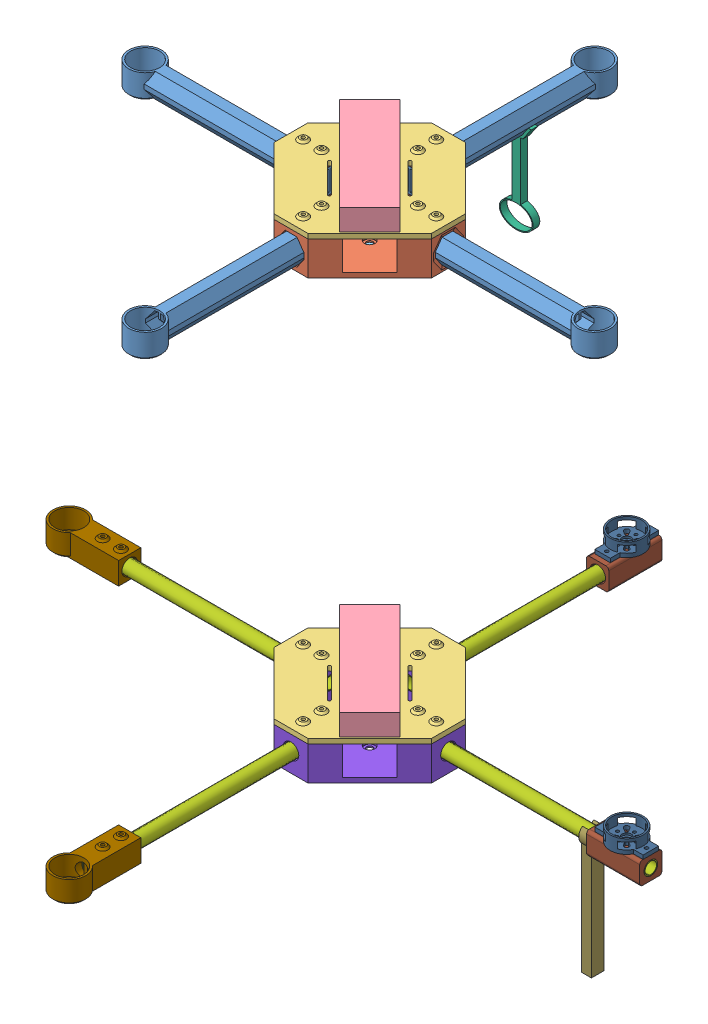
SolidWorks assembly Drone, configuration Default. Lengths in mm.
Overall size (992.84 165.03 1029.84).
269 component instances, 33 part files, 69 mates.
Components (placement in the parent):
- Braccio-1: Braccio [Default] at (4.1091 -2.9836 208.5217) size (34 25 208.52)
- Motore-1: Motore [Default] at (2.2324 -9.8606 400.0434) x (-0.70582 0 0.708391) z (-0.708391 0 -0.70582) size (268.27 83.88 262.74) (hidden)
  - D2830 - Stator-1: D2830 - Stator [Default] at (0 -2 0) x (1 0 0) z (0 1 0) size (39.17 39.17 19.95)
    - Base du stator-1: Base du stator [Default] at (0 0 2) x (0.707107 0.707107 0) z (0 0 1) size (27.7 27.7 8.01)
    - Lamelles du Stator-1: Lamelles du Stator [Default] at (0 0 10) x (0.707107 0.707107 0) z (0 0 1) size (22 22 11.74)
    - Roulement Ó billes-1: Roulement Ó billes [Default] at (0 0 2) x (0.999852 0.017205 0) z (0 0 1) size (10 10 3)
    - Bobine-1: Bobine [Default] at (3.9814 3.9814 9.9) x (0.707107 0.707107 0) z (0 0 1) size (4.61 2.4 12.14) (hidden)
    - Roulement Ó billes-2: Roulement Ó billes [Default] at (0 0 18.74) size (10 10 3)
    - Bobine-2: Bobine [Default] at (1.4573 5.4387 9.9) x (0.258819 0.965926 0) z (0 0 1) size (4.61 2.4 12.14) (hidden)
    - Bobine-3: Bobine [Default] at (-1.4573 5.4387 9.9) x (-0.258819 0.965926 0) z (0 0 1) size (4.61 2.4 12.14) (hidden)
    - Bobine-4: Bobine [Default] at (-3.9814 3.9814 9.9) x (-0.707107 0.707107 0) z (0 0 1) size (4.61 2.4 12.14) (hidden)
    - Bobine-5: Bobine [Default] at (-5.4387 1.4573 9.9) x (-0.965926 0.258819 0) z (0 0 1) size (4.61 2.4 12.14) (hidden)
    - Bobine-6: Bobine [Default] at (-5.4387 -1.4573 9.9) x (-0.965926 -0.258819 0) z (0 0 1) size (4.61 2.4 12.14) (hidden)
    - Bobine-7: Bobine [Default] at (-3.9814 -3.9814 9.9) x (-0.707107 -0.707107 0) z (0 0 1) size (4.61 2.4 12.14) (hidden)
    - Bobine-8: Bobine [Default] at (-1.4573 -5.4387 9.9) x (-0.258819 -0.965926 0) z (0 0 1) size (4.61 2.4 12.14) (hidden)
    - Bobine-9: Bobine [Default] at (1.4573 -5.4387 9.9) x (0.258819 -0.965926 0) z (0 0 1) size (4.61 2.4 12.14) (hidden)
    - Bobine-10: Bobine [Default] at (3.9814 -3.9814 9.9) x (0.707107 -0.707107 0) z (0 0 1) size (4.61 2.4 12.14) (hidden)
    - Bobine-11: Bobine [Default] at (5.4387 -1.4573 9.9) x (0.965926 -0.258819 0) z (0 0 1) size (4.61 2.4 12.14) (hidden)
    - Bobine-12: Bobine [Default] at (5.4387 1.4573 9.9) x (0.965926 0.258819 0) z (0 0 1) size (4.61 2.4 12.14) (hidden)
  - D2830 - Rotor-1: D2830 - Rotor [Default] at (-0.1467 -73.15 -0.1528) x (-0.576616 0 0.817016) z (0 1 0) size (28.2 28.2 23.5)
    - Corps supÚrieur-1: Corps supÚrieur [Default] at (0.0403 0.208 79.2501) size (28.2 28.2 23.5)
    - Goupille_M2-1: Goupille_M2 [Default] at (-4.2817 4.4914 98.5001) x (0.495514 0.49998 -0.710272) z (0.710272 -0.703927 0) size (1.7 1.7 4.5)
    - Plaque magnÚtique-1: Plaque magnÚtique [Default] at (5.2017 10.9258 80.2501) x (0.900969 -0.433884 0) z (0 0 1) size (4 1 11.5)
    - Plaque magnÚtique-2: Plaque magnÚtique [Default] at (9.3408 7.6249 80.2501) x (0.62349 -0.781831 0) z (0 0 1) size (4 1 11.5)
    - Plaque magnÚtique-3: Plaque magnÚtique [Default] at (11.6378 2.8551 80.2501) x (0.222521 -0.974928 0) z (0 0 1) size (4 1 11.5)
    - Plaque magnÚtique-4: Plaque magnÚtique [Default] at (11.6378 -2.4391 80.2501) x (-0.222521 -0.974928 0) z (0 0 1) size (4 1 11.5)
    - Plaque magnÚtique-5: Plaque magnÚtique [Default] at (9.3408 -7.2089 80.2501) x (-0.62349 -0.781831 0) z (0 0 1) size (4 1 11.5)
    - Plaque magnÚtique-6: Plaque magnÚtique [Default] at (5.2017 -10.5098 80.2501) x (-0.900969 -0.433884 0) z (0 0 1) size (4 1 11.5)
    - Plaque magnÚtique-7: Plaque magnÚtique [Default] at (0.0403 -11.6878 80.2501) x (-1 0 0) z (0 0 1) size (4 1 11.5)
    - Plaque magnÚtique-8: Plaque magnÚtique [Default] at (-5.1212 -10.5098 80.2501) x (-0.900969 0.433884 0) z (0 0 1) size (4 1 11.5)
    - Plaque magnÚtique-9: Plaque magnÚtique [Default] at (-9.2603 -7.2089 80.2501) x (-0.62349 0.781831 0) z (0 0 1) size (4 1 11.5)
    - Plaque magnÚtique-10: Plaque magnÚtique [Default] at (-11.5573 -2.4391 80.2501) x (-0.222521 0.974928 0) z (0 0 1) size (4 1 11.5)
    - Plaque magnÚtique-11: Plaque magnÚtique [Default] at (-11.5573 2.8551 80.2501) x (0.222521 0.974928 0) z (0 0 1) size (4 1 11.5)
    - Plaque magnÚtique-12: Plaque magnÚtique [Default] at (-9.2603 7.6249 80.2501) x (0.62349 0.781831 0) z (0 0 1) size (4 1 11.5)
    - Plaque magnÚtique-13: Plaque magnÚtique [Default] at (-5.1212 10.9258 80.2501) x (0.900969 0.433884 0) z (0 0 1) size (4 1 11.5)
    - Plaque magnÚtique-14: Plaque magnÚtique [Default] at (0.0403 12.1038 80.2501) size (4 1 11.5)
  - Spinner-Part1-1: Spinner-Part1 [Default] at (0 33.1 0) x (0.576616 0 -0.817016) z (0.817016 0 0.576616) size (8.94 36.28 8.94) (hidden)
  - Spinner-Part2-1: Spinner-Part2 [Default] at (0 33.1 0) x (0.576616 0 -0.817016) z (0.817016 0 0.576616) size (16 12 16) (hidden)
  - Spinner-Part3-1: Spinner-Part3 [Default] at (0 56.1 0) x (0.576616 0 -0.817016) z (0.817016 0 0.576616) size (19.01 24 18.92) (hidden)
  - Axe-1: Axe [Default] at (0 -0.9 0) x (0.964595 0 0.263735) z (0 1 0) size (3.17 3.17 45)
  - Circlip-1: Circlip [Default] at (0 -0.4 0) x (0.576616 0 -0.817016) z (0 1 0) size (5.59 4.89 0.4)
  - FAB_HELICES - 9x4.5 CCW-1: FAB_HELICES - 9x4.5 CCW [Default] at (0 50.6 0) x (-0.817016 0 -0.576616) z (0.576616 0 -0.817016) size (202.02 12.04 179) (hidden)
  - CÔble-1: CÔble [Default] at (-4.5922 4.5 -11.0866) x (-0.92388 0 0.382683) z (-0.382683 0 -0.92388) size (2.5 7.25 5.25)
  - CÔble-2: CÔble [Default] at (-8.8388 4.5 -8.8388) x (-0.707107 0 0.707107) z (-0.707107 0 -0.707107) size (2.5 7.25 5.25)
  - CÔble-3: CÔble [Default] at (-11.0866 4.5 -4.5922) x (-0.382683 0 0.92388) z (-0.92388 0 -0.382683) size (2.5 7.25 5.25)
  - CONNECTEUR - Ï3.5 - Moteur-1: CONNECTEUR - Ï3.5 - Moteur [Default] at (-80 0 -8) x (1 0 0) z (0 -1 0) size (13 5 5) (hidden)
  - CONNECTEUR - Ï3.5 - Moteur-2: CONNECTEUR - Ï3.5 - Moteur [Default] at (-80 0 0) x (1 0 0) z (0 -1 0) size (13 5 5) (hidden)
  - CONNECTEUR - Ï3.5 - Moteur-3: CONNECTEUR - Ï3.5 - Moteur [Default] at (-80 0 8) x (1 0 0) z (0 1 0) size (13 5 5) (hidden)
  - PiÞce4^RD - MOTEUR D2830 1100kv-1: PiÞce4^RD - MOTEUR D2830 1100kv [Default] at (-83.5 0 -8) x (0 -1 0) z (-1 0 0) size (5.5 5.5 13) (hidden)
  - PiÞce4^RD - MOTEUR D2830 1100kv-2: PiÞce4^RD - MOTEUR D2830 1100kv [Default] at (-83.5 0 8) x (0 -0.964264 0.264942) z (-1 0 0) size (5.5 5.5 13) (hidden)
  - PiÞce4^RD - MOTEUR D2830 1100kv-3: PiÞce4^RD - MOTEUR D2830 1100kv [Default] at (-83.5 0 0) x (0 0.521887 -0.853015) z (-1 0 0) size (5.5 5.5 13) (hidden)
  - MOTEUR - Support-1: MOTEUR - Support [Default] at (0 -1 0) x (1 0 0) z (0 -1 0) size (40 40 2) (hidden)
  - Cable_1-RD - MOTEUR D2830 1000kv-1: Cable_1-RD - MOTEUR D2830 1000kv [Default] at origin size (71.18 4.18 10.39) (hidden)
    - Cble^Cable_1-RD - MOTEUR D2830 1000kv-1: Cble^Cable_1-RD - MOTEUR D2830 1000kv [Default] at origin size (71.18 4.18 10.39)
  - Electrical_2-RD - MOTEUR D2830 1000kv-1: Electrical_2-RD - MOTEUR D2830 1000kv [Default] at origin size (74.08 7.31 25.49) (hidden)
    - Cble^Electrical_2-RD - MOTEUR D2830 1000kv-1: Cble^Electrical_2-RD - MOTEUR D2830 1000kv [Default] at origin size (74.08 7.31 25.49)
  - Cable_4-RD - MOTEUR D2830 1000kv-1: Cable_4-RD - MOTEUR D2830 1000kv [Default] at origin size (78.89 4.18 16.32) (hidden)
    - Cble^Cable_4-RD - MOTEUR D2830 1000kv-1: Cble^Cable_4-RD - MOTEUR D2830 1000kv [Default] at origin size (78.89 4.18 16.32)
  - countersunk flat head cross recess screw_iso_ISO 7046-1 - M2.5 x 6 - Z --- 6C-1: countersunk flat head cross recess screw_iso_ISO 7046-1 - M2.5 x 6 - Z --- 6C [Default] at (-8 -2 0) x (0 1 0) z (0 0 1) size (6 4.7 4.7) (hidden)
  - countersunk flat head cross recess screw_iso_ISO 7046-1 - M2.5 x 6 - Z --- 6C-2: countersunk flat head cross recess screw_iso_ISO 7046-1 - M2.5 x 6 - Z --- 6C [Default] at (0 -2 -9.5) x (0 1 0) z (0 0 1) size (6 4.7 4.7) (hidden)
  - countersunk flat head cross recess screw_iso_ISO 7046-1 - M2.5 x 6 - Z --- 6C-3: countersunk flat head cross recess screw_iso_ISO 7046-1 - M2.5 x 6 - Z --- 6C [Default] at (8 -2 0) x (0 1 0) z (0 0 1) size (6 4.7 4.7) (hidden)
  - countersunk flat head cross recess screw_iso_ISO 7046-1 - M2.5 x 6 - Z --- 6C-4: countersunk flat head cross recess screw_iso_ISO 7046-1 - M2.5 x 6 - Z --- 6C [Default] at (0 -2 9.5) x (0 1 0) z (0 0 1) size (6 4.7 4.7) (hidden)
- Corpo-1: Corpo [Default] at (-0.3221 -17.8606 224.4367) x (0.707107 0 -0.707107) z (0.707107 0 0.707107) size (140 35 140)
- Braccio-2: Braccio [Default] at (43.1166 -2.9836 165.7607) x (0 0 -1) z (1 0 0) size (34 25 208.52)
- Braccio-3: Braccio [Default] at (-38.6519 -2.7836 169.5142) x (0 0 1) z (-1 0 0) size (34 25 208.52)
- Braccio-4: Braccio [Default] at (0.3556 -2.7836 126.7532) x (-1 0 0) z (0 0 -1) size (34 25 208.52)
- Motore-2: Motore [Default] at (-230.1736 -9.6606 167.6374) x (0.708391 0 0.70582) z (-0.70582 0 0.708391) size (268.27 83.88 262.74) (hidden)
  - D2830 - Stator-1: D2830 - Stator [Default] at (0 -2 0) x (1 0 0) z (0 1 0) size (39.17 39.17 19.95)
    - Base du stator-1: Base du stator [Default] at (0 0 2) x (0.707107 0.707107 0) z (0 0 1) size (27.7 27.7 8.01)
    - Lamelles du Stator-1: Lamelles du Stator [Default] at (0 0 10) x (0.707107 0.707107 0) z (0 0 1) size (22 22 11.74)
    - Roulement Ó billes-1: Roulement Ó billes [Default] at (0 0 2) x (0.999852 0.017205 0) z (0 0 1) size (10 10 3)
    - Bobine-1: Bobine [Default] at (3.9814 3.9814 9.9) x (0.707107 0.707107 0) z (0 0 1) size (4.61 2.4 12.14) (hidden)
    - Roulement Ó billes-2: Roulement Ó billes [Default] at (0 0 18.74) size (10 10 3)
    - Bobine-2: Bobine [Default] at (1.4573 5.4387 9.9) x (0.258819 0.965926 0) z (0 0 1) size (4.61 2.4 12.14) (hidden)
    - Bobine-3: Bobine [Default] at (-1.4573 5.4387 9.9) x (-0.258819 0.965926 0) z (0 0 1) size (4.61 2.4 12.14) (hidden)
    - Bobine-4: Bobine [Default] at (-3.9814 3.9814 9.9) x (-0.707107 0.707107 0) z (0 0 1) size (4.61 2.4 12.14) (hidden)
    - Bobine-5: Bobine [Default] at (-5.4387 1.4573 9.9) x (-0.965926 0.258819 0) z (0 0 1) size (4.61 2.4 12.14) (hidden)
    - Bobine-6: Bobine [Default] at (-5.4387 -1.4573 9.9) x (-0.965926 -0.258819 0) z (0 0 1) size (4.61 2.4 12.14) (hidden)
    - Bobine-7: Bobine [Default] at (-3.9814 -3.9814 9.9) x (-0.707107 -0.707107 0) z (0 0 1) size (4.61 2.4 12.14) (hidden)
    - Bobine-8: Bobine [Default] at (-1.4573 -5.4387 9.9) x (-0.258819 -0.965926 0) z (0 0 1) size (4.61 2.4 12.14) (hidden)
    - Bobine-9: Bobine [Default] at (1.4573 -5.4387 9.9) x (0.258819 -0.965926 0) z (0 0 1) size (4.61 2.4 12.14) (hidden)
    - Bobine-10: Bobine [Default] at (3.9814 -3.9814 9.9) x (0.707107 -0.707107 0) z (0 0 1) size (4.61 2.4 12.14) (hidden)
    - Bobine-11: Bobine [Default] at (5.4387 -1.4573 9.9) x (0.965926 -0.258819 0) z (0 0 1) size (4.61 2.4 12.14) (hidden)
    - Bobine-12: Bobine [Default] at (5.4387 1.4573 9.9) x (0.965926 0.258819 0) z (0 0 1) size (4.61 2.4 12.14) (hidden)
  - D2830 - Rotor-1: D2830 - Rotor [Default] at (-0.1467 -73.15 -0.1528) x (-0.576616 0 0.817016) z (0 1 0) size (28.2 28.2 23.5)
    - Corps supÚrieur-1: Corps supÚrieur [Default] at (0.0403 0.208 79.2501) size (28.2 28.2 23.5)
    - Goupille_M2-1: Goupille_M2 [Default] at (-4.2817 4.4914 98.5001) x (0.495514 0.49998 -0.710272) z (0.710272 -0.703927 0) size (1.7 1.7 4.5)
    - Plaque magnÚtique-1: Plaque magnÚtique [Default] at (5.2017 10.9258 80.2501) x (0.900969 -0.433884 0) z (0 0 1) size (4 1 11.5)
    - Plaque magnÚtique-2: Plaque magnÚtique [Default] at (9.3408 7.6249 80.2501) x (0.62349 -0.781831 0) z (0 0 1) size (4 1 11.5)
    - Plaque magnÚtique-3: Plaque magnÚtique [Default] at (11.6378 2.8551 80.2501) x (0.222521 -0.974928 0) z (0 0 1) size (4 1 11.5)
    - Plaque magnÚtique-4: Plaque magnÚtique [Default] at (11.6378 -2.4391 80.2501) x (-0.222521 -0.974928 0) z (0 0 1) size (4 1 11.5)
    - Plaque magnÚtique-5: Plaque magnÚtique [Default] at (9.3408 -7.2089 80.2501) x (-0.62349 -0.781831 0) z (0 0 1) size (4 1 11.5)
    - Plaque magnÚtique-6: Plaque magnÚtique [Default] at (5.2017 -10.5098 80.2501) x (-0.900969 -0.433884 0) z (0 0 1) size (4 1 11.5)
    - Plaque magnÚtique-7: Plaque magnÚtique [Default] at (0.0403 -11.6878 80.2501) x (-1 0 0) z (0 0 1) size (4 1 11.5)
    - Plaque magnÚtique-8: Plaque magnÚtique [Default] at (-5.1212 -10.5098 80.2501) x (-0.900969 0.433884 0) z (0 0 1) size (4 1 11.5)
    - Plaque magnÚtique-9: Plaque magnÚtique [Default] at (-9.2603 -7.2089 80.2501) x (-0.62349 0.781831 0) z (0 0 1) size (4 1 11.5)
    - Plaque magnÚtique-10: Plaque magnÚtique [Default] at (-11.5573 -2.4391 80.2501) x (-0.222521 0.974928 0) z (0 0 1) size (4 1 11.5)
    - Plaque magnÚtique-11: Plaque magnÚtique [Default] at (-11.5573 2.8551 80.2501) x (0.222521 0.974928 0) z (0 0 1) size (4 1 11.5)
    - Plaque magnÚtique-12: Plaque magnÚtique [Default] at (-9.2603 7.6249 80.2501) x (0.62349 0.781831 0) z (0 0 1) size (4 1 11.5)
    - Plaque magnÚtique-13: Plaque magnÚtique [Default] at (-5.1212 10.9258 80.2501) x (0.900969 0.433884 0) z (0 0 1) size (4 1 11.5)
    - Plaque magnÚtique-14: Plaque magnÚtique [Default] at (0.0403 12.1038 80.2501) size (4 1 11.5)
  - Spinner-Part1-1: Spinner-Part1 [Default] at (0 33.1 0) x (0.576616 0 -0.817016) z (0.817016 0 0.576616) size (8.94 36.28 8.94) (hidden)
  - Spinner-Part2-1: Spinner-Part2 [Default] at (0 33.1 0) x (0.576616 0 -0.817016) z (0.817016 0 0.576616) size (16 12 16) (hidden)
  - Spinner-Part3-1: Spinner-Part3 [Default] at (0 56.1 0) x (0.576616 0 -0.817016) z (0.817016 0 0.576616) size (19.01 24 18.92) (hidden)
  - Axe-1: Axe [Default] at (0 -0.9 0) x (0.964595 0 0.263735) z (0 1 0) size (3.17 3.17 45)
  - Circlip-1: Circlip [Default] at (0 -0.4 0) x (0.576616 0 -0.817016) z (0 1 0) size (5.59 4.89 0.4)
  - FAB_HELICES - 9x4.5 CCW-1: FAB_HELICES - 9x4.5 CCW [Default] at (0 50.6 0) x (-0.817016 0 -0.576616) z (0.576616 0 -0.817016) size (202.02 12.04 179) (hidden)
  - CÔble-1: CÔble [Default] at (-4.5922 4.5 -11.0866) x (-0.92388 0 0.382683) z (-0.382683 0 -0.92388) size (2.5 7.25 5.25)
  - CÔble-2: CÔble [Default] at (-8.8388 4.5 -8.8388) x (-0.707107 0 0.707107) z (-0.707107 0 -0.707107) size (2.5 7.25 5.25)
  - CÔble-3: CÔble [Default] at (-11.0866 4.5 -4.5922) x (-0.382683 0 0.92388) z (-0.92388 0 -0.382683) size (2.5 7.25 5.25)
  - CONNECTEUR - Ï3.5 - Moteur-1: CONNECTEUR - Ï3.5 - Moteur [Default] at (-80 0 -8) x (1 0 0) z (0 -1 0) size (13 5 5) (hidden)
  - CONNECTEUR - Ï3.5 - Moteur-2: CONNECTEUR - Ï3.5 - Moteur [Default] at (-80 0 0) x (1 0 0) z (0 -1 0) size (13 5 5) (hidden)
  - CONNECTEUR - Ï3.5 - Moteur-3: CONNECTEUR - Ï3.5 - Moteur [Default] at (-80 0 8) x (1 0 0) z (0 1 0) size (13 5 5) (hidden)
  - PiÞce4^RD - MOTEUR D2830 1100kv-1: PiÞce4^RD - MOTEUR D2830 1100kv [Default] at (-83.5 0 -8) x (0 -1 0) z (-1 0 0) size (5.5 5.5 13) (hidden)
  - PiÞce4^RD - MOTEUR D2830 1100kv-2: PiÞce4^RD - MOTEUR D2830 1100kv [Default] at (-83.5 0 8) x (0 -0.964264 0.264942) z (-1 0 0) size (5.5 5.5 13) (hidden)
  - PiÞce4^RD - MOTEUR D2830 1100kv-3: PiÞce4^RD - MOTEUR D2830 1100kv [Default] at (-83.5 0 0) x (0 0.521887 -0.853015) z (-1 0 0) size (5.5 5.5 13) (hidden)
  - MOTEUR - Support-1: MOTEUR - Support [Default] at (0 -1 0) x (1 0 0) z (0 -1 0) size (40 40 2) (hidden)
  - Cable_1-RD - MOTEUR D2830 1000kv-1: Cable_1-RD - MOTEUR D2830 1000kv [Default] at origin size (71.18 4.18 10.39) (hidden)
    - Cble^Cable_1-RD - MOTEUR D2830 1000kv-1: Cble^Cable_1-RD - MOTEUR D2830 1000kv [Default] at origin size (71.18 4.18 10.39)
  - Electrical_2-RD - MOTEUR D2830 1000kv-1: Electrical_2-RD - MOTEUR D2830 1000kv [Default] at origin size (74.08 7.31 25.49) (hidden)
    - Cble^Electrical_2-RD - MOTEUR D2830 1000kv-1: Cble^Electrical_2-RD - MOTEUR D2830 1000kv [Default] at origin size (74.08 7.31 25.49)
  - Cable_4-RD - MOTEUR D2830 1000kv-1: Cable_4-RD - MOTEUR D2830 1000kv [Default] at origin size (78.89 4.18 16.32) (hidden)
    - Cble^Cable_4-RD - MOTEUR D2830 1000kv-1: Cble^Cable_4-RD - MOTEUR D2830 1000kv [Default] at origin size (78.89 4.18 16.32)
  - countersunk flat head cross recess screw_iso_ISO 7046-1 - M2.5 x 6 - Z --- 6C-1: countersunk flat head cross recess screw_iso_ISO 7046-1 - M2.5 x 6 - Z --- 6C [Default] at (-8 -2 0) x (0 1 0) z (0 0 1) size (6 4.7 4.7) (hidden)
  - countersunk flat head cross recess screw_iso_ISO 7046-1 - M2.5 x 6 - Z --- 6C-2: countersunk flat head cross recess screw_iso_ISO 7046-1 - M2.5 x 6 - Z --- 6C [Default] at (0 -2 -9.5) x (0 1 0) z (0 0 1) size (6 4.7 4.7) (hidden)
  - countersunk flat head cross recess screw_iso_ISO 7046-1 - M2.5 x 6 - Z --- 6C-3: countersunk flat head cross recess screw_iso_ISO 7046-1 - M2.5 x 6 - Z --- 6C [Default] at (8 -2 0) x (0 1 0) z (0 0 1) size (6 4.7 4.7) (hidden)
  - countersunk flat head cross recess screw_iso_ISO 7046-1 - M2.5 x 6 - Z --- 6C-4: countersunk flat head cross recess screw_iso_ISO 7046-1 - M2.5 x 6 - Z --- 6C [Default] at (0 -2 9.5) x (0 1 0) z (0 0 1) size (6 4.7 4.7) (hidden)
- Motore-3: Motore [Default] at (2.2324 -9.6606 -64.7685) x (-0.70582 0 0.708391) z (-0.708391 0 -0.70582) size (268.27 83.88 262.74) (hidden)
  - D2830 - Stator-1: D2830 - Stator [Default] at (0 -2 0) x (1 0 0) z (0 1 0) size (39.17 39.17 19.95)
    - Base du stator-1: Base du stator [Default] at (0 0 2) x (0.707107 0.707107 0) z (0 0 1) size (27.7 27.7 8.01)
    - Lamelles du Stator-1: Lamelles du Stator [Default] at (0 0 10) x (0.707107 0.707107 0) z (0 0 1) size (22 22 11.74)
    - Roulement Ó billes-1: Roulement Ó billes [Default] at (0 0 2) x (0.999852 0.017205 0) z (0 0 1) size (10 10 3)
    - Bobine-1: Bobine [Default] at (3.9814 3.9814 9.9) x (0.707107 0.707107 0) z (0 0 1) size (4.61 2.4 12.14) (hidden)
    - Roulement Ó billes-2: Roulement Ó billes [Default] at (0 0 18.74) size (10 10 3)
    - Bobine-2: Bobine [Default] at (1.4573 5.4387 9.9) x (0.258819 0.965926 0) z (0 0 1) size (4.61 2.4 12.14) (hidden)
    - Bobine-3: Bobine [Default] at (-1.4573 5.4387 9.9) x (-0.258819 0.965926 0) z (0 0 1) size (4.61 2.4 12.14) (hidden)
    - Bobine-4: Bobine [Default] at (-3.9814 3.9814 9.9) x (-0.707107 0.707107 0) z (0 0 1) size (4.61 2.4 12.14) (hidden)
    - Bobine-5: Bobine [Default] at (-5.4387 1.4573 9.9) x (-0.965926 0.258819 0) z (0 0 1) size (4.61 2.4 12.14) (hidden)
    - Bobine-6: Bobine [Default] at (-5.4387 -1.4573 9.9) x (-0.965926 -0.258819 0) z (0 0 1) size (4.61 2.4 12.14) (hidden)
    - Bobine-7: Bobine [Default] at (-3.9814 -3.9814 9.9) x (-0.707107 -0.707107 0) z (0 0 1) size (4.61 2.4 12.14) (hidden)
    - Bobine-8: Bobine [Default] at (-1.4573 -5.4387 9.9) x (-0.258819 -0.965926 0) z (0 0 1) size (4.61 2.4 12.14) (hidden)
    - Bobine-9: Bobine [Default] at (1.4573 -5.4387 9.9) x (0.258819 -0.965926 0) z (0 0 1) size (4.61 2.4 12.14) (hidden)
    - Bobine-10: Bobine [Default] at (3.9814 -3.9814 9.9) x (0.707107 -0.707107 0) z (0 0 1) size (4.61 2.4 12.14) (hidden)
    - Bobine-11: Bobine [Default] at (5.4387 -1.4573 9.9) x (0.965926 -0.258819 0) z (0 0 1) size (4.61 2.4 12.14) (hidden)
    - Bobine-12: Bobine [Default] at (5.4387 1.4573 9.9) x (0.965926 0.258819 0) z (0 0 1) size (4.61 2.4 12.14) (hidden)
  - D2830 - Rotor-1: D2830 - Rotor [Default] at (-0.1467 -73.15 -0.1528) x (-0.576616 0 0.817016) z (0 1 0) size (28.2 28.2 23.5)
    - Corps supÚrieur-1: Corps supÚrieur [Default] at (0.0403 0.208 79.2501) size (28.2 28.2 23.5)
    - Goupille_M2-1: Goupille_M2 [Default] at (-4.2817 4.4914 98.5001) x (0.495514 0.49998 -0.710272) z (0.710272 -0.703927 0) size (1.7 1.7 4.5)
    - Plaque magnÚtique-1: Plaque magnÚtique [Default] at (5.2017 10.9258 80.2501) x (0.900969 -0.433884 0) z (0 0 1) size (4 1 11.5)
    - Plaque magnÚtique-2: Plaque magnÚtique [Default] at (9.3408 7.6249 80.2501) x (0.62349 -0.781831 0) z (0 0 1) size (4 1 11.5)
    - Plaque magnÚtique-3: Plaque magnÚtique [Default] at (11.6378 2.8551 80.2501) x (0.222521 -0.974928 0) z (0 0 1) size (4 1 11.5)
    - Plaque magnÚtique-4: Plaque magnÚtique [Default] at (11.6378 -2.4391 80.2501) x (-0.222521 -0.974928 0) z (0 0 1) size (4 1 11.5)
    - Plaque magnÚtique-5: Plaque magnÚtique [Default] at (9.3408 -7.2089 80.2501) x (-0.62349 -0.781831 0) z (0 0 1) size (4 1 11.5)
    - Plaque magnÚtique-6: Plaque magnÚtique [Default] at (5.2017 -10.5098 80.2501) x (-0.900969 -0.433884 0) z (0 0 1) size (4 1 11.5)
    - Plaque magnÚtique-7: Plaque magnÚtique [Default] at (0.0403 -11.6878 80.2501) x (-1 0 0) z (0 0 1) size (4 1 11.5)
    - Plaque magnÚtique-8: Plaque magnÚtique [Default] at (-5.1212 -10.5098 80.2501) x (-0.900969 0.433884 0) z (0 0 1) size (4 1 11.5)
    - Plaque magnÚtique-9: Plaque magnÚtique [Default] at (-9.2603 -7.2089 80.2501) x (-0.62349 0.781831 0) z (0 0 1) size (4 1 11.5)
    - Plaque magnÚtique-10: Plaque magnÚtique [Default] at (-11.5573 -2.4391 80.2501) x (-0.222521 0.974928 0) z (0 0 1) size (4 1 11.5)
    - Plaque magnÚtique-11: Plaque magnÚtique [Default] at (-11.5573 2.8551 80.2501) x (0.222521 0.974928 0) z (0 0 1) size (4 1 11.5)
    - Plaque magnÚtique-12: Plaque magnÚtique [Default] at (-9.2603 7.6249 80.2501) x (0.62349 0.781831 0) z (0 0 1) size (4 1 11.5)
    - Plaque magnÚtique-13: Plaque magnÚtique [Default] at (-5.1212 10.9258 80.2501) x (0.900969 0.433884 0) z (0 0 1) size (4 1 11.5)
    - Plaque magnÚtique-14: Plaque magnÚtique [Default] at (0.0403 12.1038 80.2501) size (4 1 11.5)
  - Spinner-Part1-1: Spinner-Part1 [Default] at (0 33.1 0) x (0.576616 0 -0.817016) z (0.817016 0 0.576616) size (8.94 36.28 8.94) (hidden)
  - Spinner-Part2-1: Spinner-Part2 [Default] at (0 33.1 0) x (0.576616 0 -0.817016) z (0.817016 0 0.576616) size (16 12 16) (hidden)
  - Spinner-Part3-1: Spinner-Part3 [Default] at (0 56.1 0) x (0.576616 0 -0.817016) z (0.817016 0 0.576616) size (19.01 24 18.92) (hidden)
  - Axe-1: Axe [Default] at (0 -0.9 0) x (0.964595 0 0.263735) z (0 1 0) size (3.17 3.17 45)
  - Circlip-1: Circlip [Default] at (0 -0.4 0) x (0.576616 0 -0.817016) z (0 1 0) size (5.59 4.89 0.4)
  - FAB_HELICES - 9x4.5 CCW-1: FAB_HELICES - 9x4.5 CCW [Default] at (0 50.6 0) x (-0.817016 0 -0.576616) z (0.576616 0 -0.817016) size (202.02 12.04 179) (hidden)
  - CÔble-1: CÔble [Default] at (-4.5922 4.5 -11.0866) x (-0.92388 0 0.382683) z (-0.382683 0 -0.92388) size (2.5 7.25 5.25)
  - CÔble-2: CÔble [Default] at (-8.8388 4.5 -8.8388) x (-0.707107 0 0.707107) z (-0.707107 0 -0.707107) size (2.5 7.25 5.25)
  - CÔble-3: CÔble [Default] at (-11.0866 4.5 -4.5922) x (-0.382683 0 0.92388) z (-0.92388 0 -0.382683) size (2.5 7.25 5.25)
  - CONNECTEUR - Ï3.5 - Moteur-1: CONNECTEUR - Ï3.5 - Moteur [Default] at (-80 0 -8) x (1 0 0) z (0 -1 0) size (13 5 5) (hidden)
  - CONNECTEUR - Ï3.5 - Moteur-2: CONNECTEUR - Ï3.5 - Moteur [Default] at (-80 0 0) x (1 0 0) z (0 -1 0) size (13 5 5) (hidden)
  - CONNECTEUR - Ï3.5 - Moteur-3: CONNECTEUR - Ï3.5 - Moteur [Default] at (-80 0 8) x (1 0 0) z (0 1 0) size (13 5 5) (hidden)
  - PiÞce4^RD - MOTEUR D2830 1100kv-1: PiÞce4^RD - MOTEUR D2830 1100kv [Default] at (-83.5 0 -8) x (0 -1 0) z (-1 0 0) size (5.5 5.5 13) (hidden)
  - PiÞce4^RD - MOTEUR D2830 1100kv-2: PiÞce4^RD - MOTEUR D2830 1100kv [Default] at (-83.5 0 8) x (0 -0.964264 0.264942) z (-1 0 0) size (5.5 5.5 13) (hidden)
  - PiÞce4^RD - MOTEUR D2830 1100kv-3: PiÞce4^RD - MOTEUR D2830 1100kv [Default] at (-83.5 0 0) x (0 0.521887 -0.853015) z (-1 0 0) size (5.5 5.5 13) (hidden)
  - MOTEUR - Support-1: MOTEUR - Support [Default] at (0 -1 0) x (1 0 0) z (0 -1 0) size (40 40 2) (hidden)
  - Cable_1-RD - MOTEUR D2830 1000kv-1: Cable_1-RD - MOTEUR D2830 1000kv [Default] at origin size (71.18 4.18 10.39) (hidden)
    - Cble^Cable_1-RD - MOTEUR D2830 1000kv-1: Cble^Cable_1-RD - MOTEUR D2830 1000kv [Default] at origin size (71.18 4.18 10.39)
  - Electrical_2-RD - MOTEUR D2830 1000kv-1: Electrical_2-RD - MOTEUR D2830 1000kv [Default] at origin size (74.08 7.31 25.49) (hidden)
    - Cble^Electrical_2-RD - MOTEUR D2830 1000kv-1: Cble^Electrical_2-RD - MOTEUR D2830 1000kv [Default] at origin size (74.08 7.31 25.49)
  - Cable_4-RD - MOTEUR D2830 1000kv-1: Cable_4-RD - MOTEUR D2830 1000kv [Default] at origin size (78.89 4.18 16.32) (hidden)
    - Cble^Cable_4-RD - MOTEUR D2830 1000kv-1: Cble^Cable_4-RD - MOTEUR D2830 1000kv [Default] at origin size (78.89 4.18 16.32)
  - countersunk flat head cross recess screw_iso_ISO 7046-1 - M2.5 x 6 - Z --- 6C-1: countersunk flat head cross recess screw_iso_ISO 7046-1 - M2.5 x 6 - Z --- 6C [Default] at (-8 -2 0) x (0 1 0) z (0 0 1) size (6 4.7 4.7) (hidden)
  - countersunk flat head cross recess screw_iso_ISO 7046-1 - M2.5 x 6 - Z --- 6C-2: countersunk flat head cross recess screw_iso_ISO 7046-1 - M2.5 x 6 - Z --- 6C [Default] at (0 -2 -9.5) x (0 1 0) z (0 0 1) size (6 4.7 4.7) (hidden)
  - countersunk flat head cross recess screw_iso_ISO 7046-1 - M2.5 x 6 - Z --- 6C-3: countersunk flat head cross recess screw_iso_ISO 7046-1 - M2.5 x 6 - Z --- 6C [Default] at (8 -2 0) x (0 1 0) z (0 0 1) size (6 4.7 4.7) (hidden)
  - countersunk flat head cross recess screw_iso_ISO 7046-1 - M2.5 x 6 - Z --- 6C-4: countersunk flat head cross recess screw_iso_ISO 7046-1 - M2.5 x 6 - Z --- 6C [Default] at (0 -2 9.5) x (0 1 0) z (0 0 1) size (6 4.7 4.7) (hidden)
- Motore-4: Motore [Default] at (234.6384 -9.8606 167.6374) x (0.708391 0 0.70582) z (-0.70582 0 0.708391) size (268.27 83.88 262.74) (hidden)
  - D2830 - Stator-1: D2830 - Stator [Default] at (0 -2 0) x (1 0 0) z (0 1 0) size (39.17 39.17 19.95)
    - Base du stator-1: Base du stator [Default] at (0 0 2) x (0.707107 0.707107 0) z (0 0 1) size (27.7 27.7 8.01)
    - Lamelles du Stator-1: Lamelles du Stator [Default] at (0 0 10) x (0.707107 0.707107 0) z (0 0 1) size (22 22 11.74)
    - Roulement Ó billes-1: Roulement Ó billes [Default] at (0 0 2) x (0.999852 0.017205 0) z (0 0 1) size (10 10 3)
    - Bobine-1: Bobine [Default] at (3.9814 3.9814 9.9) x (0.707107 0.707107 0) z (0 0 1) size (4.61 2.4 12.14) (hidden)
    - Roulement Ó billes-2: Roulement Ó billes [Default] at (0 0 18.74) size (10 10 3)
    - Bobine-2: Bobine [Default] at (1.4573 5.4387 9.9) x (0.258819 0.965926 0) z (0 0 1) size (4.61 2.4 12.14) (hidden)
    - Bobine-3: Bobine [Default] at (-1.4573 5.4387 9.9) x (-0.258819 0.965926 0) z (0 0 1) size (4.61 2.4 12.14) (hidden)
    - Bobine-4: Bobine [Default] at (-3.9814 3.9814 9.9) x (-0.707107 0.707107 0) z (0 0 1) size (4.61 2.4 12.14) (hidden)
    - Bobine-5: Bobine [Default] at (-5.4387 1.4573 9.9) x (-0.965926 0.258819 0) z (0 0 1) size (4.61 2.4 12.14) (hidden)
    - Bobine-6: Bobine [Default] at (-5.4387 -1.4573 9.9) x (-0.965926 -0.258819 0) z (0 0 1) size (4.61 2.4 12.14) (hidden)
    - Bobine-7: Bobine [Default] at (-3.9814 -3.9814 9.9) x (-0.707107 -0.707107 0) z (0 0 1) size (4.61 2.4 12.14) (hidden)
    - Bobine-8: Bobine [Default] at (-1.4573 -5.4387 9.9) x (-0.258819 -0.965926 0) z (0 0 1) size (4.61 2.4 12.14) (hidden)
    - Bobine-9: Bobine [Default] at (1.4573 -5.4387 9.9) x (0.258819 -0.965926 0) z (0 0 1) size (4.61 2.4 12.14) (hidden)
    - Bobine-10: Bobine [Default] at (3.9814 -3.9814 9.9) x (0.707107 -0.707107 0) z (0 0 1) size (4.61 2.4 12.14) (hidden)
    - Bobine-11: Bobine [Default] at (5.4387 -1.4573 9.9) x (0.965926 -0.258819 0) z (0 0 1) size (4.61 2.4 12.14) (hidden)
    - Bobine-12: Bobine [Default] at (5.4387 1.4573 9.9) x (0.965926 0.258819 0) z (0 0 1) size (4.61 2.4 12.14) (hidden)
  - D2830 - Rotor-1: D2830 - Rotor [Default] at (-0.1467 -73.15 -0.1528) x (-0.576616 0 0.817016) z (0 1 0) size (28.2 28.2 23.5)
    - Corps supÚrieur-1: Corps supÚrieur [Default] at (0.0403 0.208 79.2501) size (28.2 28.2 23.5)
    - Goupille_M2-1: Goupille_M2 [Default] at (-4.2817 4.4914 98.5001) x (0.495514 0.49998 -0.710272) z (0.710272 -0.703927 0) size (1.7 1.7 4.5)
    - Plaque magnÚtique-1: Plaque magnÚtique [Default] at (5.2017 10.9258 80.2501) x (0.900969 -0.433884 0) z (0 0 1) size (4 1 11.5)
    - Plaque magnÚtique-2: Plaque magnÚtique [Default] at (9.3408 7.6249 80.2501) x (0.62349 -0.781831 0) z (0 0 1) size (4 1 11.5)
    - Plaque magnÚtique-3: Plaque magnÚtique [Default] at (11.6378 2.8551 80.2501) x (0.222521 -0.974928 0) z (0 0 1) size (4 1 11.5)
    - Plaque magnÚtique-4: Plaque magnÚtique [Default] at (11.6378 -2.4391 80.2501) x (-0.222521 -0.974928 0) z (0 0 1) size (4 1 11.5)
    - Plaque magnÚtique-5: Plaque magnÚtique [Default] at (9.3408 -7.2089 80.2501) x (-0.62349 -0.781831 0) z (0 0 1) size (4 1 11.5)
    - Plaque magnÚtique-6: Plaque magnÚtique [Default] at (5.2017 -10.5098 80.2501) x (-0.900969 -0.433884 0) z (0 0 1) size (4 1 11.5)
    - Plaque magnÚtique-7: Plaque magnÚtique [Default] at (0.0403 -11.6878 80.2501) x (-1 0 0) z (0 0 1) size (4 1 11.5)
    - Plaque magnÚtique-8: Plaque magnÚtique [Default] at (-5.1212 -10.5098 80.2501) x (-0.900969 0.433884 0) z (0 0 1) size (4 1 11.5)
    - Plaque magnÚtique-9: Plaque magnÚtique [Default] at (-9.2603 -7.2089 80.2501) x (-0.62349 0.781831 0) z (0 0 1) size (4 1 11.5)
    - Plaque magnÚtique-10: Plaque magnÚtique [Default] at (-11.5573 -2.4391 80.2501) x (-0.222521 0.974928 0) z (0 0 1) size (4 1 11.5)
    - Plaque magnÚtique-11: Plaque magnÚtique [Default] at (-11.5573 2.8551 80.2501) x (0.222521 0.974928 0) z (0 0 1) size (4 1 11.5)
    - Plaque magnÚtique-12: Plaque magnÚtique [Default] at (-9.2603 7.6249 80.2501) x (0.62349 0.781831 0) z (0 0 1) size (4 1 11.5)
    - Plaque magnÚtique-13: Plaque magnÚtique [Default] at (-5.1212 10.9258 80.2501) x (0.900969 0.433884 0) z (0 0 1) size (4 1 11.5)
    - Plaque magnÚtique-14: Plaque magnÚtique [Default] at (0.0403 12.1038 80.2501) size (4 1 11.5)
  - Spinner-Part1-1: Spinner-Part1 [Default] at (0 33.1 0) x (0.576616 0 -0.817016) z (0.817016 0 0.576616) size (8.94 36.28 8.94) (hidden)
  - Spinner-Part2-1: Spinner-Part2 [Default] at (0 33.1 0) x (0.576616 0 -0.817016) z (0.817016 0 0.576616) size (16 12 16) (hidden)
  - Spinner-Part3-1: Spinner-Part3 [Default] at (0 56.1 0) x (0.576616 0 -0.817016) z (0.817016 0 0.576616) size (19.01 24 18.92) (hidden)
  - Axe-1: Axe [Default] at (0 -0.9 0) x (0.964595 0 0.263735) z (0 1 0) size (3.17 3.17 45)
  - Circlip-1: Circlip [Default] at (0 -0.4 0) x (0.576616 0 -0.817016) z (0 1 0) size (5.59 4.89 0.4)
  - FAB_HELICES - 9x4.5 CCW-1: FAB_HELICES - 9x4.5 CCW [Default] at (0 50.6 0) x (-0.817016 0 -0.576616) z (0.576616 0 -0.817016) size (202.02 12.04 179) (hidden)
  - CÔble-1: CÔble [Default] at (-4.5922 4.5 -11.0866) x (-0.92388 0 0.382683) z (-0.382683 0 -0.92388) size (2.5 7.25 5.25)
  - CÔble-2: CÔble [Default] at (-8.8388 4.5 -8.8388) x (-0.707107 0 0.707107) z (-0.707107 0 -0.707107) size (2.5 7.25 5.25)
  - CÔble-3: CÔble [Default] at (-11.0866 4.5 -4.5922) x (-0.382683 0 0.92388) z (-0.92388 0 -0.382683) size (2.5 7.25 5.25)
  - CONNECTEUR - Ï3.5 - Moteur-1: CONNECTEUR - Ï3.5 - Moteur [Default] at (-80 0 -8) x (1 0 0) z (0 -1 0) size (13 5 5) (hidden)
  - CONNECTEUR - Ï3.5 - Moteur-2: CONNECTEUR - Ï3.5 - Moteur [Default] at (-80 0 0) x (1 0 0) z (0 -1 0) size (13 5 5) (hidden)
  - CONNECTEUR - Ï3.5 - Moteur-3: CONNECTEUR - Ï3.5 - Moteur [Default] at (-80 0 8) x (1 0 0) z (0 1 0) size (13 5 5) (hidden)
  - PiÞce4^RD - MOTEUR D2830 1100kv-1: PiÞce4^RD - MOTEUR D2830 1100kv [Default] at (-83.5 0 -8) x (0 -1 0) z (-1 0 0) size (5.5 5.5 13) (hidden)
  - PiÞce4^RD - MOTEUR D2830 1100kv-2: PiÞce4^RD - MOTEUR D2830 1100kv [Default] at (-83.5 0 8) x (0 -0.964264 0.264942) z (-1 0 0) size (5.5 5.5 13) (hidden)
  - PiÞce4^RD - MOTEUR D2830 1100kv-3: PiÞce4^RD - MOTEUR D2830 1100kv [Default] at (-83.5 0 0) x (0 0.521887 -0.853015) z (-1 0 0) size (5.5 5.5 13) (hidden)
  - MOTEUR - Support-1: MOTEUR - Support [Default] at (0 -1 0) x (1 0 0) z (0 -1 0) size (40 40 2) (hidden)
  - Cable_1-RD - MOTEUR D2830 1000kv-1: Cable_1-RD - MOTEUR D2830 1000kv [Default] at origin size (71.18 4.18 10.39) (hidden)
    - Cble^Cable_1-RD - MOTEUR D2830 1000kv-1: Cble^Cable_1-RD - MOTEUR D2830 1000kv [Default] at origin size (71.18 4.18 10.39)
  - Electrical_2-RD - MOTEUR D2830 1000kv-1: Electrical_2-RD - MOTEUR D2830 1000kv [Default] at origin size (74.08 7.31 25.49) (hidden)
    - Cble^Electrical_2-RD - MOTEUR D2830 1000kv-1: Cble^Electrical_2-RD - MOTEUR D2830 1000kv [Default] at origin size (74.08 7.31 25.49)
  - Cable_4-RD - MOTEUR D2830 1000kv-1: Cable_4-RD - MOTEUR D2830 1000kv [Default] at origin size (78.89 4.18 16.32) (hidden)
    - Cble^Cable_4-RD - MOTEUR D2830 1000kv-1: Cble^Cable_4-RD - MOTEUR D2830 1000kv [Default] at origin size (78.89 4.18 16.32)
  - countersunk flat head cross recess screw_iso_ISO 7046-1 - M2.5 x 6 - Z --- 6C-1: countersunk flat head cross recess screw_iso_ISO 7046-1 - M2.5 x 6 - Z --- 6C [Default] at (-8 -2 0) x (0 1 0) z (0 0 1) size (6 4.7 4.7) (hidden)
  - countersunk flat head cross recess screw_iso_ISO 7046-1 - M2.5 x 6 - Z --- 6C-2: countersunk flat head cross recess screw_iso_ISO 7046-1 - M2.5 x 6 - Z --- 6C [Default] at (0 -2 -9.5) x (0 1 0) z (0 0 1) size (6 4.7 4.7) (hidden)
  - countersunk flat head cross recess screw_iso_ISO 7046-1 - M2.5 x 6 - Z --- 6C-3: countersunk flat head cross recess screw_iso_ISO 7046-1 - M2.5 x 6 - Z --- 6C [Default] at (8 -2 0) x (0 1 0) z (0 0 1) size (6 4.7 4.7) (hidden)
  - countersunk flat head cross recess screw_iso_ISO 7046-1 - M2.5 x 6 - Z --- 6C-4: countersunk flat head cross recess screw_iso_ISO 7046-1 - M2.5 x 6 - Z --- 6C [Default] at (0 -2 9.5) x (0 1 0) z (0 0 1) size (6 4.7 4.7) (hidden)
- Coperchio_sopra-1: Coperchio_sopra [Default] at (-1.0904 17.1394 108.6054) x (0.707107 0 0.707107) z (-0.707107 0 0.707107) size (140 7 140)
- Batteria-1: Batteria [Default] at (-7.2092 22.1394 164.6214) x (0.707107 0 0.707107) z (-0.707107 0 0.707107) size (137 22 44)
- sony_mout-1: sony_mout [Default] at (-2.4108 -31.8606 157.2868) x (-0.707107 0 0.707107) z (-0.707107 0 -0.707107) size (75 22.43 75)
- Piedino-1: Piedino [Default] at (7.9789 -27.0022 9.1425) size (35 97.08 7)
- Braccio_carbonio-1: Braccio_carbonio [Default] at (457.1519 -2.1993 661.0701) size (14 14 250)
- Braccio_carbonio-2: Braccio_carbonio [Default] at (458.1906 -1.4304 329.3015) x (0.965228 0.261408 0) z (0 0 1) size (14 14 250)
- Braccio_carbonio-3: Braccio_carbonio [Default] at (413.8964 6.5715 618.2043) x (0 0.088695 -0.996059) z (-1 0 0) size (14 14 250)
- Braccio_carbonio-4: Braccio_carbonio [Default] at (495.665 -2.1993 617.8146) x (0 0 -1) z (1 0 0) size (14 14 250)
- Corpo_tubi_carbon-1: Corpo_tubi_carbon [Default] at (452.2262 -17.8606 676.9851) x (0.707107 0 -0.707107) z (0.707107 0 0.707107) size (140 35 140)
- Posaggio_motore-1: Posaggio_motore [Default] at (458.3318 -0.2236 868.5501) size (34 25 79.52)
- Posaggio_motore-2: Posaggio_motore [Default] at (206.4164 -0.2236 623.7369) x (0 0 1) z (-1 0 0) size (34 25 79.52)
- Coperchio_sopra-2: Coperchio_sopra [Default] at (451.4579 17.1394 561.1538) x (0.707107 0 0.707107) z (-0.707107 0 0.707107) size (140 7 140)
- Batteria-2: Batteria [Default] at (445.3392 22.1394 617.1698) x (0.707107 0 0.707107) z (-0.707107 0 0.707107) size (137 22 44)
- Posaggio_motore_2-1: Posaggio_motore_2 [Default] at (670.6649 20.2942 620.0121) x (0 0 -1) z (1 0 0) size (34 37 55)
  - Bicchiere_motore-1: Bicchiere_motore [Default] at (-0.1736 -6.7048 50) size (34 14 50)
  - Posaggio_motore_2-1: Posaggio_motore_2 [Default] at (3.3774 -20.5178 20) size (23 23 55)
- Posaggio_motore_2-2: Posaggio_motore_2 [Default] at (454.6071 20.2942 404.3016) x (-1 0 0) z (0 0 -1) size (34 37 55)
  - Bicchiere_motore-1: Bicchiere_motore [Default] at (-0.1736 -6.7048 50) size (34 14 50)
  - Posaggio_motore_2-1: Posaggio_motore_2 [Default] at (3.3774 -20.5178 20) size (23 23 55)
- Piedino_tondo-1: Piedino_tondo [Default] at (690.665 -38.5422 625.4823) x (0 0 1) z (0 -1 0) size (19.3 10 130.7)
Mates (geometry in assembly coordinates):
- Coincidente1: coincident anti-aligned: plane of Braccio-1 through (2.2324 -9.8606 400.0434) normal (0 1 0); plane of Motore-1/D2830 - Stator-1/Base du stator-1 through (2.2324 -9.8606 400.0434) normal (0 -1 0)
- Concentrico1: concentric aligned: circle of Braccio-1; circle of Motore-1/D2830 - Stator-1/Roulement Ó billes-1
- Parallelo1: parallel anti-aligned: plane of Braccio-1 through (4.1091 12.1394 388.5217) normal (0 1 0); plane of Corpo-1 through (7.8324 12.2394 266.6324) normal (0 -1 0)
- Distanza1: distance = 0.1 mm anti-aligned: plane of Braccio-1 through (4.1091 12.1394 388.5217) normal (0 1 0); plane of Corpo-1 through (7.8324 12.2394 266.6324) normal (0 -1 0)
- Distanza2: distance = 0.1 mm anti-aligned: plane of Braccio-1 through (14.7324 -2.9836 388.5217) normal (1 0 0); plane of Corpo-1 through (14.8324 2.2394 266.6324) normal (-1 0 0)
- Coincidente8: coincident aligned: plane of Braccio-1 through (4.1091 -2.9836 208.5217) normal (0 0 -1); plane of Corpo-1 through (14.8324 -12.9606 208.5217) normal (0 0 -1)
- Distanza4: distance = 0.1 mm anti-aligned: plane of Braccio-2 through (223.1166 12.1394 165.7607) normal (0 1 0); plane of Corpo-1 through (-96.7626 12.2394 173.2374) normal (0 -1 0)
- Distanza5: distance = 0.1 mm anti-aligned: plane of Braccio-2 through (223.1166 -2.9836 180.1374) normal (0 0 1); plane of Corpo-1 through (-96.7626 2.2394 180.2374) normal (0 0 -1)
- Coincidente14: coincident aligned: plane of Corpo-1 through (43.1166 -12.9606 155.0374) normal (-1 0 0); plane of Braccio-2 through (43.1166 -2.9836 165.7607) normal (-1 0 0)
- Distanza6: distance = 0.1 mm anti-aligned: plane of Braccio-3 through (-218.6519 12.3394 169.5142) normal (0 1 0); plane of Corpo-1 through (-96.7626 12.2394 173.2374) normal (0 -1 0)
- Distanza7: distance = 0.1 mm anti-aligned: plane of Braccio-3 through (-218.6519 -2.7836 180.1374) normal (0 0 1); plane of Corpo-1 through (-96.7626 2.2394 180.2374) normal (0 0 -1)
- Coincidente17: coincident aligned: plane of Corpo-1 through (-38.6519 -12.9606 180.2374) normal (1 0 0); plane of Braccio-3 through (-38.6519 -2.7836 169.5142) normal (1 0 0)
- Distanza8: distance = 0.1 mm anti-aligned: plane of Braccio-4 through (0.3556 12.3394 -53.2468) normal (0 1 0); plane of Corpo-1 through (7.8324 12.2394 266.6324) normal (0 -1 0)
- Distanza9: distance = 0.1 mm anti-aligned: plane of Braccio-4 through (-10.2676 -2.7836 -53.2468) normal (-1 0 0); plane of Corpo-1 through (-10.3676 2.2394 266.6324) normal (1 0 0)
- Coincidente20: coincident aligned: plane of Corpo-1 through (-10.3676 -12.9606 126.7532) normal (0 0 1); plane of Braccio-4 through (0.3556 -2.7836 126.7532) normal (0 0 1)
- Coincidente21: coincident anti-aligned: plane of Braccio-2 through (234.6384 -9.8606 167.6374) normal (0 1 0); plane of Motore-4/D2830 - Stator-1/Base du stator-1 through (234.6384 -9.8606 167.6374) normal (0 -1 0)
- Concentrico2: concentric aligned: circle of Braccio-2; circle of Motore-4/D2830 - Stator-1/Roulement Ó billes-1
- Concentrico3: concentric anti-aligned: circle of Braccio-2; circle of Motore-4/D2830 - Stator-1/Base du stator-1
- Coincidente22: coincident anti-aligned: plane of Braccio-4 through (2.2324 -9.6606 -64.7685) normal (0 1 0); plane of Motore-3/D2830 - Stator-1/Base du stator-1 through (2.2324 -9.6606 -64.7685) normal (0 -1 0)
- Concentrico4: concentric anti-aligned: circle of Braccio-4; circle of Motore-3/D2830 - Stator-1/Roulement Ó billes-1
- Coincidente23: coincident anti-aligned: plane of Braccio-3 through (-230.1736 -9.6606 167.6374) normal (0 1 0); plane of Motore-2/D2830 - Stator-1/Base du stator-1 through (-230.1736 -9.6606 167.6374) normal (0 -1 0)
- Concentrico6: concentric anti-aligned: circle of Braccio-3; circle of Motore-2/D2830 - Stator-1/Base du stator-1
- Concentrico7: concentric aligned: circle of Braccio-3; circle of Motore-2/D2830 - Stator-1/Roulement Ó billes-1
- Coincidente24: coincident anti-aligned: plane of Corpo-1 through (-0.3221 17.1394 224.4367) normal (0 1 0); plane of Coperchio_sopra-1 through (-1.0904 17.1394 108.6054) normal (0 -1 0)
- Coincidente25: coincident anti-aligned: line of Corpo-1 through (19.7324 17.1394 86.1425) axis (-1 0 0); line of Coperchio_sopra-1 through (-15.2676 17.1394 86.1425) axis (1 0 0)
- Coincidente26: coincident anti-aligned: line of Corpo-1 through (83.7273 17.1394 185.1374) axis (0 0 -1); line of Coperchio_sopra-1 through (83.7273 17.1394 150.1374) axis (0 0 1)
- Parallelo2: parallel aligned: plane of Batteria-1 through (-30.6481 44.1394 103.6443) normal (-0.707107 0 -0.707107); plane of Coperchio_sopra-1 through (2.2324 22.1394 68.6425) normal (-0.707107 0 -0.707107)
- Coincidente28: coincident anti-aligned: plane of Coperchio_sopra-1 through (-1.0904 22.1394 108.6054) normal (0 1 0); plane of Batteria-1 through (-7.2092 22.1394 164.6214) normal (0 -1 0)
- Distanza10: distance = 48 mm aligned: plane of Batteria-1 through (-61.7608 44.1394 134.757) normal (-0.707107 0 0.707107); plane of Coperchio_sopra-1 through (-96.7626 22.1394 167.6374) normal (-0.707107 0 0.707107)
- Distanza11: distance = 1.5 mm aligned: plane of Batteria-1 through (66.2255 44.1394 200.5179) normal (0.707107 0 0.707107); plane of Coperchio_sopra-1 through (101.2273 22.1394 167.6374) normal (0.707107 0 0.707107)
- Concentrico8: concentric anti-aligned: circle of Corpo-1; circle of sony_mout-1
- Parallelo3: parallel aligned: line of Corpo-1 through (-79.2626 -17.8606 185.1374) axis (0.707107 0 0.707107); line of sony_mout-1 through (-24.285 -31.8606 151.7267) axis (0.707107 0 0.707107)
- Distanza12: distance = 9 mm anti-aligned: plane of Corpo-1 through (-0.3221 -17.8606 224.4367) normal (0 -1 0); plane of sony_mout-1 through (23.4447 -26.8606 146.4234) normal (0 1 0)
- Coincidente29: coincident anti-aligned: plane of Braccio-4 through (0.3556 -12.6606 -53.2468) normal (0 -1 0); plane of Piedino-1 through (7.9789 -12.6606 16.1425) normal (0 1 0)
- Distanza14: distance = 0.1 mm: line of Braccio-4 through (14.7324 -2.6606 -53.2468) axis (0 0 1); plane of Piedino-1 through (1.1582 -22.2281 16.1425) normal (-0.819252 0.573433 0)
- Coincidente33: coincident aligned: plane of Braccio_carbonio-2 through (454.7807 2.0894 579.3015) normal (0 0 1); plane of Corpo_tubi_carbon-1 through (442.1807 -12.9606 579.3015) normal (0 0 1)
- Concentrico10: concentric aligned: circle of Braccio_carbonio-2; circle of Corpo_tubi_carbon-1
- Concentrico11: concentric anti-aligned: circle of Braccio_carbonio-3; circle of Corpo_tubi_carbon-1
- Coincidente34: coincident aligned: plane of Braccio_carbonio-3 through (413.8964 2.0894 620.1858) normal (1 0 0); plane of Corpo_tubi_carbon-1 through (413.8964 -12.9606 632.7858) normal (1 0 0)
- Coincidente36: coincident aligned: plane of Corpo-1 through (-0.3221 -17.8606 224.4367) normal (0 -1 0); plane of Corpo_tubi_carbon-1 through (452.2262 -17.8606 676.9851) normal (0 -1 0)
- Coincidente37: coincident aligned: plane of Corpo-1 through (-15.2676 17.1394 249.1324) normal (-0.707107 0 0.707107); plane of Corpo_tubi_carbon-1 through (437.2807 17.1394 701.6807) normal (-0.707107 0 0.707107)
- Distanza20: distance = 500 mm anti-aligned: plane of Corpo_tubi_carbon-1 through (373.2858 17.1394 602.6858) normal (-0.707107 0 -0.707107); plane of Corpo-1 through (83.7273 17.1394 185.1374) normal (0.707107 0 0.707107)
- Concentrico12: concentric anti-aligned: circle of Braccio_carbonio-1; circle of Corpo_tubi_carbon-1
- Coincidente39: coincident aligned: plane of Braccio_carbonio-1 through (454.7807 2.0894 661.0701) normal (0 0 -1); plane of Corpo_tubi_carbon-1 through (467.3807 -12.9606 661.0701) normal (0 0 -1)
- Concentrico13: concentric anti-aligned: circle of Braccio_carbonio-4; circle of Corpo_tubi_carbon-1
- Coincidente40: coincident aligned: plane of Braccio_carbonio-4 through (495.665 2.0894 620.1858) normal (-1 0 0); plane of Corpo_tubi_carbon-1 through (495.665 -12.9606 607.5858) normal (-1 0 0)
- Coincidente41: coincident anti-aligned: plane of Braccio_carbonio-1 through (454.7807 2.0894 911.0701) normal (0 0 1); plane of Posaggio_motore-1 through (452.7807 -9.4106 911.0701) normal (0 0 -1)
- Concentrico14: concentric anti-aligned: circle of Braccio_carbonio-1; circle of Posaggio_motore-1
- Coincidente43: coincident anti-aligned: plane of Braccio_carbonio-3 through (163.8964 2.0894 620.1858) normal (-1 0 0); plane of Posaggio_motore-2 through (163.8964 -9.4106 618.1858) normal (1 0 0)
- Concentrico16: concentric anti-aligned: circle of Braccio_carbonio-3; circle of Posaggio_motore-2
- Parallelo8: parallel aligned: plane of Corpo_tubi_carbon-1 through (452.2262 17.1394 676.9851) normal (0 1 0); plane of Posaggio_motore-1 through (458.3318 13.5894 918.5501) normal (0 1 0)
- Parallelo9: parallel aligned: plane of Corpo_tubi_carbon-1 through (452.2262 17.1394 676.9851) normal (0 1 0); plane of Posaggio_motore-2 through (156.4164 13.5894 623.7369) normal (0 1 0)
- Coincidente45: coincident anti-aligned: line of Corpo_tubi_carbon-1 through (437.2807 17.1394 701.6807) axis (1 0 0); line of Coperchio_sopra-2 through (472.2807 17.1394 701.6807) axis (-1 0 0)
- Coincidente47: coincident anti-aligned: line of Corpo_tubi_carbon-1 through (472.2807 17.1394 538.6908) axis (-1 0 0); line of Coperchio_sopra-2 through (437.2807 17.1394 538.6908) axis (1 0 0)
- Coincidente48: coincident anti-aligned: line of Corpo_tubi_carbon-1 through (536.2757 17.1394 637.6858) axis (0 0 -1); line of Coperchio_sopra-2 through (536.2757 17.1394 602.6858) axis (0 0 1)
- Parallelo10: parallel aligned: plane of Batteria-1 through (66.2255 44.1394 200.5179) normal (0.707107 0 0.707107); plane of Batteria-2 through (518.7739 44.1394 653.0663) normal (0.707107 0 0.707107)
- Coincidente50: coincident anti-aligned: plane of Coperchio_sopra-2 through (451.4579 22.1394 561.1538) normal (0 1 0); plane of Batteria-2 through (445.3392 22.1394 617.1698) normal (0 -1 0)
- Coincidente51: coincident aligned: plane of Batteria-1 through (-30.6481 44.1394 103.6443) normal (0.707107 0 -0.707107); plane of Batteria-2 through (421.9002 44.1394 556.1926) normal (0.707107 0 -0.707107)
- Distanza21: distance = 1.5 mm: line of Coperchio_sopra-2 through (437.2807 22.1394 538.6908) axis (-0.707107 0 0.707107); line of Batteria-2 through (421.9002 22.1394 556.1926) axis (-0.707107 0 0.707107)
- Concentrico17: concentric aligned: circle of Braccio_carbonio-2; circle of Posaggio_motore_2-2/Posaggio_motore_2-1
- Coincidente52: coincident aligned: plane of Braccio_carbonio-2 through (454.7807 2.0894 329.3015) normal (0 0 -1); plane of Posaggio_motore_2-2/Posaggio_motore_2-1 through (451.2296 -0.2236 329.3015) normal (0 0 -1)
- Concentrico18: concentric aligned: circle of Braccio_carbonio-4; circle of Posaggio_motore_2-1/Posaggio_motore_2-1
- Coincidente53: coincident aligned: plane of Braccio_carbonio-4 through (745.665 2.0894 620.1858) normal (1 0 0); plane of Posaggio_motore_2-1/Posaggio_motore_2-1 through (745.665 -0.2236 616.6347) normal (1 0 0)
- Parallelo11: parallel aligned: plane of Coperchio_sopra-2 through (451.4579 22.1394 561.1538) normal (0 1 0); plane of Posaggio_motore_2-1/Posaggio_motore_2-1 through (745.665 13.5894 616.6347) normal (0 1 0)
- Parallelo12: parallel aligned: plane of Coperchio_sopra-2 through (451.4579 22.1394 561.1538) normal (0 1 0); plane of Posaggio_motore_2-2/Posaggio_motore_2-1 through (451.2296 13.5894 329.3015) normal (0 1 0)
- Parallelo13: parallel anti-aligned: plane of Coperchio_sopra-2 through (451.4579 22.1394 561.1538) normal (0 1 0); plane of Piedino_tondo-1 through (674.6408 -120.8893 625.4823) normal (0 -1 0)
- Parallelo14: parallel anti-aligned: plane of Posaggio_motore_2-1/Posaggio_motore_2-1 through (745.665 -0.2236 616.6347) normal (1 0 0); plane of Piedino_tondo-1 through (674.6408 -38.5422 625.4823) normal (-1 0 0)
- Concentrico19: concentric anti-aligned: cylinder of Braccio_carbonio-4 through (745.665 2.0894 620.1858) axis (-1 0 0) radius 7; cylinder of Piedino_tondo-1 through (674.6408 2.0894 620.1858) axis (1 0 0) radius 7.15
- Coincidente56: coincident anti-aligned: plane of Posaggio_motore_2-1/Posaggio_motore_2-1 through (690.665 -0.2236 616.6347) normal (-1 0 0); plane of Piedino_tondo-1 through (690.665 -38.5422 625.4823) normal (1 0 0)
